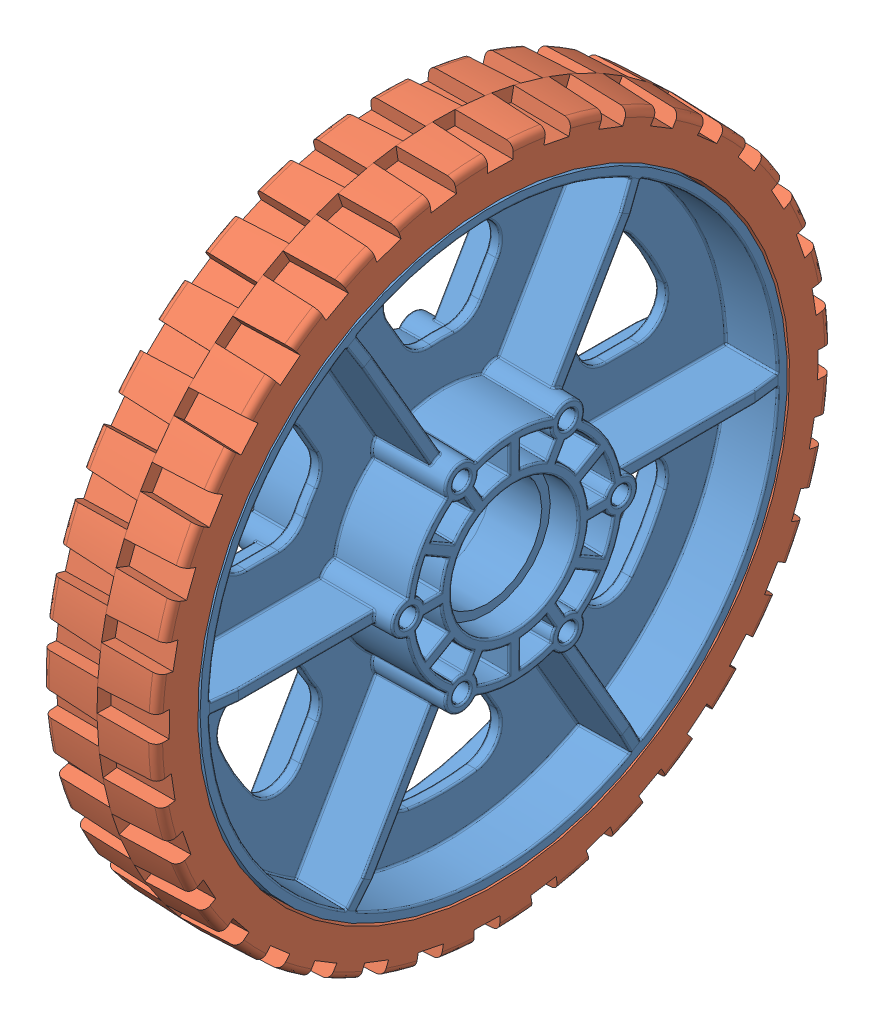
SolidWorks assembly 1250-20-D0003, configuration Default. Lengths in mm.
Overall size (34.93 200.99 200.99).
2 component instances, 2 part files, 1 mates.
Components (placement in the parent):
- 6 wheel Rev 4-1: 6 wheel Rev 4 [Default] at (51.8682 83.819 89.9109) size (34.93 132.08 132.08)
- 6 wheel tread II-1: 6 wheel tread II [Default] at (39.1682 83.819 89.9109) x (0 0.404147 -0.914694) z (1 0 0) size (152.4 152.4 25.58)
Mates (geometry in assembly coordinates):
- Concentric1: concentric: cone of 6 wheel Rev 4-1 through (51.8682 83.819 89.9109) axis (1 0 0); cone of 6 wheel tread II-1 through (51.8682 83.819 89.9109) axis (1 0 0)
